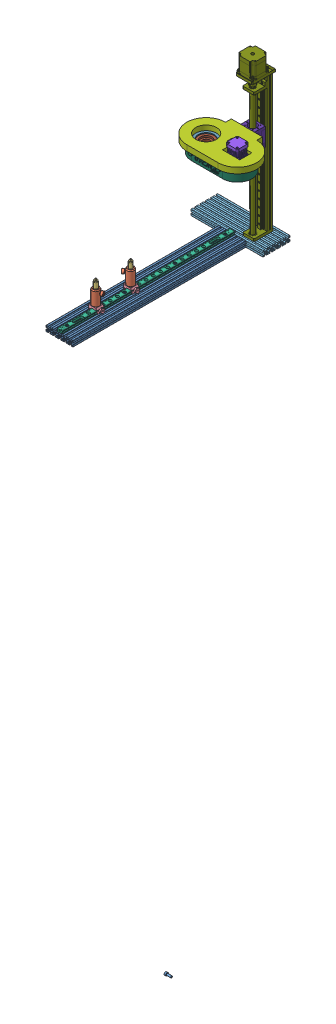
SolidWorks assembly OpenCALAssembly.v3.2, configuration Default. Lengths in mm.
Overall size (733.87 2470.14 969.59).
44 component instances, 19 part files, 57 mates.
Components (placement in the parent):
- 20-2020-Black-25-CL.stp-1: 20-2020-Black-25-CL.stp [Default] at (5.4558 13.0651 39.4201) size (94 20 600)
- PH50_M-Solidworks-1: PH50_M-Solidworks [Default] at (39.4918 57.7304 -95.7663) x (-0.331511 0 -0.943451) z (0.943451 0 -0.331511) size (25 50.44 35.14)
- TR75_M-Solidworks-1: TR75_M-Solidworks [Default] at (34.6119 36.3776 -93.7876) x (0.8365 0 0.547967) z (-0.547967 0 0.8365) size (12.67 80.02 12.87)
- RC1-Solidworks-1: RC1-Solidworks [Default] at (53.5095 23.0651 -81.0876) x (0 0 -1) z (1 0 0) size (25.4 16.53 39.23)
- 20-2020-Black-25-CLShort.stp-1: 20-2020-Black-25-CLShort.stp [Default] at (148.2574 13.0651 -570.5799) x (0 0 -1) z (1 0 0) size (94 20 250)
- PH50_M-Solidworks-2: PH50_M-Solidworks [Default] at (30.7203 57.7304 -211.3859) x (0.637938 0 0.770088) z (-0.770088 0 0.637938) size (25 50.44 35.14)
- TR75_M-Solidworks-2: TR75_M-Solidworks [Default] at (34.6119 34.7631 -214.9333) x (0.31409 0 0.949393) z (-0.949393 0 0.31409) size (12.67 80.02 12.87)
- RC1-Solidworks-2: RC1-Solidworks [Default] at (53.5095 23.0651 -202.2333) x (0 0 -1) z (1 0 0) size (25.4 16.53 39.23)
- RLA600_M-Solidworks-1: RLA600_M-Solidworks [Default] at (42.6639 28.1451 -260.6859) size (19.05 9.53 600)
- OpenCAL Assembly v3.2-1: OpenCAL Assembly v3.2 [Default] at (101.0074 1571.532 -1444.6393) x (0.001711 0 -0.999999) z (-0.999999 0 -0.001711) size (155.19 106 243.36)
  - RotationStage-1: RotationStage [Default] at (-945.7806 1212.3177 20.6963) x (1 0 0) z (0 0 1) size (155.19 80 243.36)
  - Stepper with GT2 Pulley and Closed-Loop Belt-1: Stepper with GT2 Pulley and Closed-Loop Belt [Default] at (-979.0617 1273.6406 62.5787) x (-0.000327 0 1) z (1 0 0.000327) size (166.51 64.5 74)
    - Copy of Assem2^Stepper with GT2 Pulley and Closed-Loop Belt-1: Copy of Assem2^Stepper with GT2 Pulley and Closed-Loop Belt [Default] at origin size (47.8 64.5 42.3) (virtual)
      - Nema17-1: Nema17 [Predeterminado] at (-104.7481 84.323 13.4322) x (0 0 1) z (1 0 0) size (42.3 64.5 47.8)
      - T5 Pulley-1: T5 Pulley [Predeterminado] at (-104.7481 37.623 13.4322) x (0 -1 0) z (0 0 1) size (14.8 16 16)
    - Belt-1: Belt [Default] at (-108.6865 25.623 13.493) size (153.36 6 74)
  - Collet with Gear and Toolholder-1: Collet with Gear and Toolholder [Default] at (-962.1619 1275.7752 52.9156) x (-1 0 -0.00041) z (-0.00041 0 1) size (98.27 60.66 98.27)
    - er32 x 34ths ToolHolderOpenCAL-1: er32 x 34ths ToolHolderOpenCAL [Default] at (-15.7823 32.6902 -13.7293) x (0.420729 0 0.907186) z (0.907186 0 -0.420729) size (74 44.7 74)
    - ER32 COLLET NUT-1: ER32 COLLET NUT [Default] at (3.8533 13.4515 11.5736) x (0 -1 0) z (0.99027 0 0.13916) size (22.61 50 50)
    - ER32-20.step-1: ER32-20.step [Default] at (3.6132 -14.2638 13.2822) x (0.698361 0 0.715746) z (0 -1 0) size (32.96 32.96 40.01)
    - BallBearing-1: BallBearing [Default] at (3.6132 11.6902 13.2822) x (0.999353 0 0.035955) z (-0.035955 0 0.999353) size (72 9 72)
    - BallBearing-2: BallBearing [Default] at (3.6132 46.3902 13.2822) x (-0.871455 0 -0.490475) z (-0.490475 0 0.871455) size (72 9 72)
  - Rotation Stage Bottom Plate-1: Rotation Stage Bottom Plate [Default] at (-965.7806 1232.3176 66.1963) x (-0.010268 0 -0.999947) z (0.999947 0 -0.010268) size (210.35 36.77 133.14)
- ZStageAssm-2: ZStageAssm [Default] at (487.3353 488.304 -911.4771) x (0 -1 0) z (-1 0 0) size (562.65 93.47 86.84)
  - FSL40E350-BC-B57-1: FSL40E350-BC-B57 [Default] at (78.5613 293.4958 501.3397) size (562.65 93.47 86.84)
  - ZCarriage-1: ZCarriage [Default] at (-181.088 293.4958 501.3397) size (67.97 49.14 48.01)
- T-Nut 20 M5 v1.step-1: T-Nut 20 M5 v1.step [Default] at (42.6639 23.0651 14.3141) x (0 0 1) z (-1 0 0) size (10 4.5 9.24)
- socket head cap screw_am1-19: socket head cap screw_am1 [B18.3.1M - 5 x 0.8 x 8 Hex SHCS -- 8NHX] at (42.6639 30.6051 14.3141) x (0 -1 0) z (0 0 1) size (13 8.5 8.5)
- socket head cap screw_am1-20: socket head cap screw_am1 [B18.3.1M - 5 x 0.8 x 8 Hex SHCS -- 8NHX] at (42.6639 30.6051 -535.6859) x (0 -1 0) z (0 0 1) size (13 8.5 8.5)
- socket head cap screw_am1-21: socket head cap screw_am1 [B18.3.1M - 5 x 0.8 x 8 Hex SHCS -- 8NHX] at (42.6639 30.6051 -360.6859) x (0 -1 0) z (0 0 1) size (13 8.5 8.5)
- socket head cap screw_am1-22: socket head cap screw_am1 [B18.3.1M - 5 x 0.8 x 8 Hex SHCS -- 8NHX] at (42.6639 30.6051 -185.6859) x (0 -1 0) z (0 0 1) size (13 8.5 8.5)
- socket head cap screw_am1-23: socket head cap screw_am1 [B18.3.1M - 3 x 0.5 x 10 Hex SHCS -- 10NHX] at (156.9985 336.2143 -463.4519) x (0 1 0) z (0 0 1) size (13 5.5 5.5)
- socket head cap screw_am1-24: socket head cap screw_am1 [B18.3.1M - 3 x 0.5 x 10 Hex SHCS -- 10NHX] at (157.0414 336.2143 -494.4519) x (0 1 0) z (0 0 1) size (13 5.5 5.5)
- socket head cap screw_am1-25: socket head cap screw_am1 [B18.3.1M - 3 x 0.5 x 10 Hex SHCS -- 10NHX] at (126.0415 336.2143 -494.4948) x (0 1 0) z (0 0 1) size (13 5.5 5.5)
- socket head cap screw_am1-26: socket head cap screw_am1 [B18.3.1M - 3 x 0.5 x 10 Hex SHCS -- 10NHX] at (125.9985 336.2143 -463.4948) x (0 1 0) z (0 0 1) size (13 5.5 5.5)
- socket head cap screw_am1-27: socket head cap screw_am1 [B18.3.1M - 6 x 1.0 x 20 Hex SHCS -- 20NHX] at (97.1413 316.7143 -546.4733) x (0 0 -1) z (1 0 0) size (26 10 10)
- socket head cap screw_am1-28: socket head cap screw_am1 [B18.3.1M - 6 x 1.0 x 20 Hex SHCS -- 20NHX] at (77.1413 316.7143 -546.4733) x (0 0 -1) z (1 0 0) size (26 10 10)
- socket head cap screw_am1-29: socket head cap screw_am1 [B18.3.1M - 6 x 1.0 x 20 Hex SHCS -- 20NHX] at (97.1413 331.7143 -546.4733) x (0 0 -1) z (1 0 0) size (26 10 10)
- socket head cap screw_am1-30: socket head cap screw_am1 [B18.3.1M - 6 x 1.0 x 20 Hex SHCS -- 20NHX] at (77.1413 331.7143 -546.4733) x (0 0 -1) z (1 0 0) size (26 10 10)
- socket head cap screw_am1-31: socket head cap screw_am1 [B18.3.1M - 6 x 1.0 x 16 Hex SHCS -- 16NHX] at (316.7296 -1814.5075 -53.5357) size (22 10 10)
- socket head cap screw_am1-32: socket head cap screw_am1 [B18.3.1M - 6 x 1.0 x 16 Hex SHCS -- 16NHX] at (135.6103 328.2143 -537.5447) x (0 1 0) z (0 0 1) size (22 10 10)
- socket head cap screw_am1-33: socket head cap screw_am1 [B18.3.1M - 6 x 1.0 x 16 Hex SHCS -- 16NHX] at (39.2479 328.2143 -420.5457) x (0 1 0) z (0 0 1) size (22 10 10)
- socket head cap screw_am1-34: socket head cap screw_am1 [B18.3.1M - 6 x 1.0 x 16 Hex SHCS -- 16NHX] at (39.2479 328.2143 -537.4009) x (0 1 0) z (0 0 1) size (22 10 10)
- socket head cap screw_am1-35: socket head cap screw_am1 [B18.3.1M - 6 x 1.0 x 16 Hex SHCS -- 16NHX] at (135.4097 328.2143 -420.3812) x (0 1 0) z (0 0 1) size (22 10 10)
Mates (geometry in assembly coordinates):
- Concentric1: concentric aligned: circle of PH50_M-Solidworks-1; cylinder of TR75_M-Solidworks-1 through (34.6119 111.3838 -93.7876) axis (0 1 0) radius 6.3373
- Concentric2: concentric anti-aligned: circle of PH50_M-Solidworks-1; circle of RC1-Solidworks-1
- Coincident4: coincident anti-aligned: plane of PH50_M-Solidworks-1 through (43.7754 38.5591 -67.7092) normal (0 -1 0); plane of RC1-Solidworks-1 through (21.9119 38.5591 -81.0876) normal (0 1 0)
- Parallel1: parallel aligned: plane of 20-2020-Black-25-CL.stp-1 through (-3.0442 4.5651 39.4201) normal (0 0 1); plane of RC1-Solidworks-1 through (21.9119 23.0651 -81.0876) normal (0 0 1)
- Coincident6: coincident aligned: line of 20-2020-Black-25-CL.stp-1 through (45.5938 23.0651 -560.5799) axis (0 0 1); line of RC1-Solidworks-1 through (45.5938 23.0651 -106.4876) axis (0 0 1)
- Coincident7: coincident anti-aligned: plane of 20-2020-Black-25-CL.stp-1 through (32.4558 23.0651 14.4201) normal (0 1 0); plane of RC1-Solidworks-1 through (21.9119 23.0651 -81.0876) normal (0 -1 0)
- Coincident13: coincident anti-aligned: plane of 20-2020-Black-25-CL.stp-1 through (89.4558 4.5651 14.4201) normal (1 0 0); plane of 20-2020-Black-25-CL.stp-3 through (89.4558 13.0651 -350.9237) normal (-1 0 0)
- Concentric3: concentric aligned: circle of PH50_M-Solidworks-2; cylinder of TR75_M-Solidworks-2 through (34.6119 109.7693 -214.9333) axis (0 1 0) radius 6.3373
- Concentric4: concentric anti-aligned: circle of PH50_M-Solidworks-2; circle of RC1-Solidworks-2
- Coincident21: coincident anti-aligned: plane of PH50_M-Solidworks-2 through (16.9784 38.5591 -236.2196) normal (0 -1 0); plane of RC1-Solidworks-2 through (21.9119 38.5591 -202.2333) normal (0 1 0)
- Parallel2: parallel aligned: plane of 20-2020-Black-25-CL.stp-1 through (-3.0442 4.5651 39.4201) normal (0 0 1); plane of RC1-Solidworks-2 through (21.9119 23.0651 -202.2333) normal (0 0 1)
- Coincident22: coincident aligned: line of 20-2020-Black-25-CL.stp-1 through (45.5938 23.0651 -560.5799) axis (0 0 1); line of RC1-Solidworks-2 through (45.5938 23.0651 -227.6333) axis (0 0 1)
- Coincident23: coincident anti-aligned: plane of 20-2020-Black-25-CL.stp-1 through (32.4558 23.0651 14.4201) normal (0 1 0); plane of RC1-Solidworks-2 through (21.9119 23.0651 -202.2333) normal (0 -1 0)
- Parallel4: parallel anti-aligned: line of 20-2020-Black-25-CL.stp-1 through (50.9558 23.0651 39.4201) axis (-1 0 0); line of RLA600_M-Solidworks-1 through (36.3393 23.3191 39.3141) axis (1 0 0)
- Coincident28: coincident anti-aligned: plane of 20-2020-Black-25-CL.stp-1 through (50.9558 23.0651 14.4201) normal (0 1 0); plane of RLA600_M-Solidworks-1 through (52.1889 23.0651 39.3141) normal (0 -1 0)
- Coincident34: coincident aligned: plane of 20-2020-Black-25-CL.stp-1 through (57.8178 23.0651 14.4201) normal (0 1 0); plane of 20-2020-Black-25-CLShort.stp-1 through (123.2574 23.0651 -567.4419) normal (0 1 0)
- Coincident35: coincident anti-aligned: plane of 20-2020-Black-25-CL.stp-1 through (5.4558 13.0651 -560.5799) normal (0 0 -1); plane of 20-2020-Black-25-CLShort.stp-1 through (123.2574 21.5651 -560.5799) normal (0 0 1)
- Coincident36: coincident anti-aligned: plane of 20-2020-Black-25-CLShort.stp-1 through (123.2574 23.0651 -641.4419) normal (0 1 0); plane of ZStageAssm-2/FSL40E350-BC-B57-1 through (87.1413 23.0651 -604.1733) normal (0 -1 0)
- Parallel5: parallel aligned: plane of 20-2020-Black-25-CLShort.stp-1 through (148.2574 4.5651 -562.0799) normal (1 0 0); plane of ZStageAssm-2/FSL40E350-BC-B57-1 through (107.1413 23.0651 -636.6733) normal (1 0 0)
- Concentric13: concentric anti-aligned: circle of OpenCAL Assembly v3.2-1/RotationStage-1; cylinder of ZStageAssm-2/ZCarriage-1 through (97.1413 316.7143 -566.4733) axis (0 0 1) radius 3
- Parallel8: parallel anti-aligned: plane of OpenCAL Assembly v3.2-1/RotationStage-1 through (141.52 359.2143 -566.4733) normal (1 0 0); plane of ZStageAssm-2/ZCarriage-1 through (111.1412 291.7143 -586.5733) normal (-1 0 0)
- Coincident42: coincident aligned: plane of OpenCAL Assembly v3.2-1/RotationStage-1 through (78.6927 359.2143 -566.4733) normal (0 0 -1); plane of ZStageAssm-2/ZCarriage-1 through (111.1413 356.7143 -566.4733) normal (0 0 -1)
- Concentric14: concentric aligned: cylinder of OpenCAL Assembly v3.2-1/Rotation Stage Bottom Plate-1 through (135.6103 329.2143 -537.5447) axis (0 -1 0) radius 2.9; cylinder of socket head cap screw_am-3 through (135.6103 296.4643 -537.5447) axis (0 -1 0) radius 5
- Coincident43: coincident anti-aligned: plane of OpenCAL Assembly v3.2-1/Rotation Stage Bottom Plate-1 through (135.6152 334.2143 -540.4447) normal (0 -1 0); plane of socket head cap screw_am-3 through (130.6103 334.2143 -537.5447) normal (0 1 0)
- Concentric15: concentric aligned: cylinder of OpenCAL Assembly v3.2-1/Rotation Stage Bottom Plate-1 through (39.2479 329.2143 -420.5457) axis (0 -1 0) radius 5; cylinder of socket head cap screw_am-4 through (39.2479 296.4643 -420.5457) axis (0 -1 0) radius 5
- Coincident44: coincident anti-aligned: plane of OpenCAL Assembly v3.2-1/Rotation Stage Bottom Plate-1 through (39.2529 334.2143 -423.4457) normal (0 -1 0); plane of socket head cap screw_am-4 through (34.2479 334.2143 -420.5457) normal (0 1 0)
- Concentric16: concentric aligned: cylinder of OpenCAL Assembly v3.2-1/Rotation Stage Bottom Plate-1 through (39.2479 329.2143 -537.4009) axis (0 -1 0) radius 2.9; cylinder of socket head cap screw_am-5 through (39.2479 296.4643 -537.4009) axis (0 -1 0) radius 5
- Coincident45: coincident anti-aligned: plane of OpenCAL Assembly v3.2-1/Rotation Stage Bottom Plate-1 through (39.2529 334.2143 -540.3009) normal (0 -1 0); plane of socket head cap screw_am-5 through (34.2479 334.2143 -537.4009) normal (0 1 0)
- Concentric17: concentric aligned: cylinder of OpenCAL Assembly v3.2-1/Rotation Stage Bottom Plate-1 through (135.4097 329.2143 -420.3812) axis (0 -1 0) radius 2.9; cylinder of socket head cap screw_am-6 through (135.4097 296.4643 -420.3812) axis (0 -1 0) radius 5
- Coincident46: coincident anti-aligned: plane of OpenCAL Assembly v3.2-1/Rotation Stage Bottom Plate-1 through (135.4147 334.2143 -423.2812) normal (0 -1 0); plane of socket head cap screw_am-6 through (130.4097 334.2143 -420.3812) normal (0 1 0)
- Concentric22: concentric aligned: cylinder of OpenCAL Assembly v3.2-1/RotationStage-1 through (97.1413 316.7143 -546.4733) axis (0 0 1) radius 5.5; cylinder of socket head cap screw_am-11 through (97.1413 316.7143 -514.7233) axis (0 0 1) radius 5
- Coincident51: coincident anti-aligned: plane of OpenCAL Assembly v3.2-1/RotationStage-1 through (94.6664 314.2394 -552.4733) normal (0 0 1); plane of socket head cap screw_am-11 through (97.1413 321.7143 -552.4733) normal (0 0 -1)
- Concentric23: concentric aligned: cylinder of OpenCAL Assembly v3.2-1/RotationStage-1 through (77.1413 316.7143 -546.4733) axis (0 0 1) radius 3.5; cylinder of socket head cap screw_am-12 through (77.1413 316.7143 -514.7233) axis (0 0 1) radius 5
- Coincident52: coincident anti-aligned: plane of OpenCAL Assembly v3.2-1/RotationStage-1 through (74.6664 314.2394 -552.4733) normal (0 0 1); plane of socket head cap screw_am-12 through (77.1413 321.7143 -552.4733) normal (0 0 -1)
- Concentric24: concentric aligned: cylinder of OpenCAL Assembly v3.2-1/RotationStage-1 through (97.1413 331.7143 -546.4733) axis (0 0 1) radius 3.5; cylinder of socket head cap screw_am-13 through (97.1413 331.7143 -514.7233) axis (0 0 1) radius 5
- Coincident53: coincident anti-aligned: plane of OpenCAL Assembly v3.2-1/RotationStage-1 through (94.6664 329.2394 -552.4733) normal (0 0 1); plane of socket head cap screw_am-13 through (97.1413 336.7143 -552.4733) normal (0 0 -1)
- Concentric25: concentric aligned: cylinder of OpenCAL Assembly v3.2-1/RotationStage-1 through (77.1413 331.7143 -546.4733) axis (0 0 1) radius 3.5; cylinder of socket head cap screw_am-14 through (77.1413 331.7143 -514.7233) axis (0 0 1) radius 5
- Coincident54: coincident anti-aligned: plane of OpenCAL Assembly v3.2-1/RotationStage-1 through (74.6664 329.2394 -552.4733) normal (0 0 1); plane of socket head cap screw_am-14 through (77.1413 336.7143 -552.4733) normal (0 0 -1)
- Concentric26: concentric anti-aligned: cylinder of OpenCAL Assembly v3.2-1/Stepper with GT2 Pulley and Closed-Loop Belt-1/Copy of Assem2^Stepper with GT2 Pulley and Closed-Loop Belt-1/Nema17-1 through (156.9985 385.2143 -463.4519) axis (0 1 0) radius 1.6; cylinder of socket head cap screw_am-15 through (156.9985 304.4643 -463.4519) axis (0 -1 0) radius 2.75
- Coincident55: coincident anti-aligned: plane of OpenCAL Assembly v3.2-1/RotationStage-1 through (78.6927 339.2143 -498.8954) normal (0 -1 0); plane of socket head cap screw_am-15 through (154.2485 339.2143 -463.4519) normal (0 1 0)
- Concentric27: concentric anti-aligned: cylinder of OpenCAL Assembly v3.2-1/Stepper with GT2 Pulley and Closed-Loop Belt-1/Copy of Assem2^Stepper with GT2 Pulley and Closed-Loop Belt-1/Nema17-1 through (157.0414 385.2143 -494.4519) axis (0 1 0) radius 1.6; cylinder of socket head cap screw_am-16 through (157.0414 304.4643 -494.4519) axis (0 -1 0) radius 2.75
- Coincident56: coincident anti-aligned: plane of OpenCAL Assembly v3.2-1/RotationStage-1 through (78.6927 339.2143 -498.8954) normal (0 -1 0); plane of socket head cap screw_am-16 through (154.2914 339.2143 -494.4519) normal (0 1 0)
- Concentric28: concentric anti-aligned: cylinder of OpenCAL Assembly v3.2-1/Stepper with GT2 Pulley and Closed-Loop Belt-1/Copy of Assem2^Stepper with GT2 Pulley and Closed-Loop Belt-1/Nema17-1 through (126.0415 385.2143 -494.4948) axis (0 1 0) radius 1.6; cylinder of socket head cap screw_am-17 through (126.0415 304.4643 -494.4948) axis (0 -1 0) radius 2.75
- Coincident57: coincident anti-aligned: plane of OpenCAL Assembly v3.2-1/RotationStage-1 through (78.6927 339.2143 -498.8954) normal (0 -1 0); plane of socket head cap screw_am-17 through (123.2915 339.2143 -494.4948) normal (0 1 0)
- Concentric29: concentric anti-aligned: cylinder of OpenCAL Assembly v3.2-1/Stepper with GT2 Pulley and Closed-Loop Belt-1/Copy of Assem2^Stepper with GT2 Pulley and Closed-Loop Belt-1/Nema17-1 through (125.9985 385.2143 -463.4948) axis (0 1 0) radius 1.6; cylinder of socket head cap screw_am-18 through (125.9985 304.4643 -463.4948) axis (0 -1 0) radius 2.75
- Coincident58: coincident anti-aligned: plane of OpenCAL Assembly v3.2-1/RotationStage-1 through (78.6927 339.2143 -498.8954) normal (0 -1 0); plane of socket head cap screw_am-18 through (123.2485 339.2143 -463.4948) normal (0 1 0)
- Concentric30: concentric aligned: cylinder of RLA600_M-Solidworks-1 through (42.6639 32.3361 14.3141) axis (0 1 0) radius 3.3655; cylinder of socket head cap screw_am-19 through (42.6639 62.3551 14.3141) axis (0 1 0) radius 4.25
- Coincident59: coincident anti-aligned: plane of RLA600_M-Solidworks-1 through (46.0294 25.6051 14.3141) normal (0 1 0); plane of socket head cap screw_am-19 through (46.9139 25.6051 14.3141) normal (0 -1 0)
- Concentric31: concentric aligned: cylinder of RLA600_M-Solidworks-1 through (42.6639 32.3361 -535.6859) axis (0 1 0) radius 3.3655; cylinder of socket head cap screw_am-20 through (42.6639 62.3551 -535.6859) axis (0 1 0) radius 4.25
- Coincident60: coincident anti-aligned: plane of RLA600_M-Solidworks-1 through (46.0294 25.6051 -535.6859) normal (0 1 0); plane of socket head cap screw_am-20 through (46.9139 25.6051 -535.6859) normal (0 -1 0)
- Concentric32: concentric aligned: cylinder of RLA600_M-Solidworks-1 through (42.6639 32.3361 -360.6859) axis (0 1 0) radius 3.3655; cylinder of socket head cap screw_am-21 through (42.6639 62.3551 -360.6859) axis (0 1 0) radius 4.25
- Coincident61: coincident anti-aligned: plane of RLA600_M-Solidworks-1 through (46.0294 25.6051 -360.6859) normal (0 1 0); plane of socket head cap screw_am-21 through (46.9139 25.6051 -360.6859) normal (0 -1 0)
- Concentric33: concentric aligned: cylinder of RLA600_M-Solidworks-1 through (42.6639 32.3361 -185.6859) axis (0 1 0) radius 3.3655; cylinder of socket head cap screw_am-22 through (42.6639 62.3551 -185.6859) axis (0 1 0) radius 4.25
- Coincident62: coincident anti-aligned: plane of RLA600_M-Solidworks-1 through (46.0294 25.6051 -185.6859) normal (0 1 0); plane of socket head cap screw_am-22 through (46.9139 25.6051 -185.6859) normal (0 -1 0)
- Concentric34: concentric anti-aligned: cylinder of socket head cap screw_am-19 through (42.6639 62.3551 14.3141) axis (0 1 0) radius 2.5; circle of T-Nut 20 M5 v1.step-1
- Parallel9: parallel: line of 20-2020-Black-25-CL.stp-1 through (48.4508 20.3313 -560.5799) axis (0 0 1); plane of T-Nut 20 M5 v1.step-1 through (39.6639 22.9651 14.3141) normal (-1 0 0)
- Coincident64: coincident anti-aligned: plane of 20-2020-Black-25-CL.stp-1 through (36.9688 21.5651 14.4201) normal (0 -1 0); plane of T-Nut 20 M5 v1.step-1 through (39.6639 21.5651 14.3141) normal (0 1 0)
